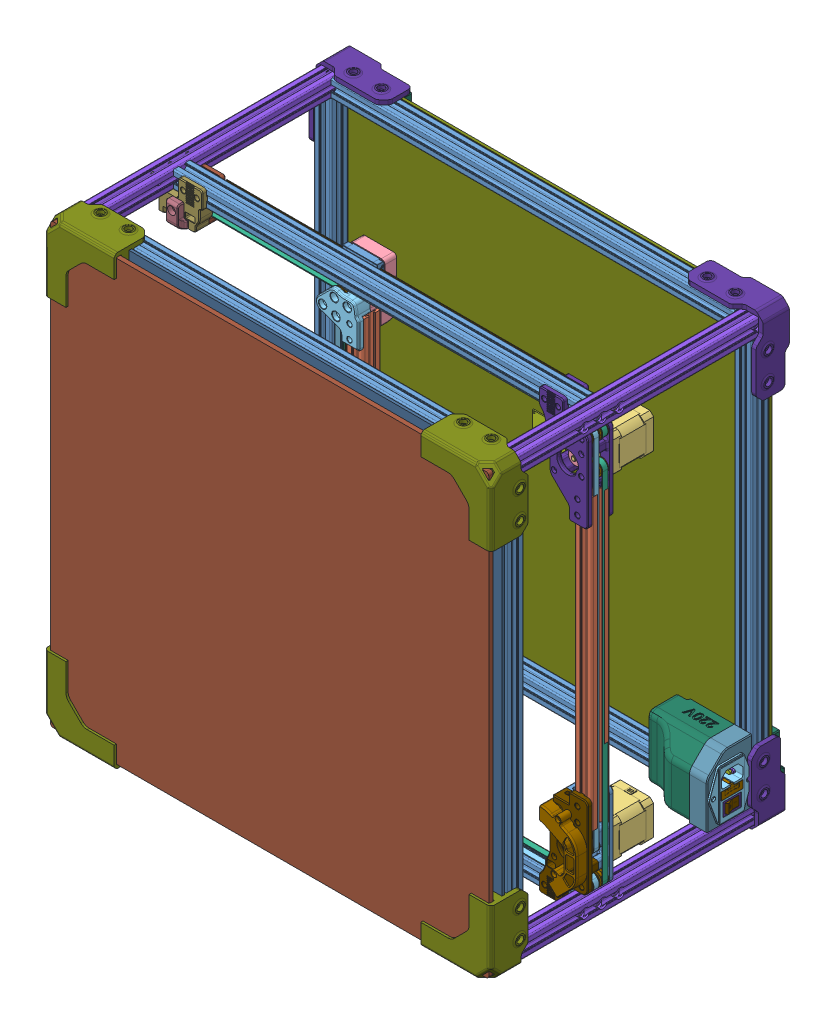
SolidWorks assembly Assem, configuration Default. Lengths in mm.
Overall size (512.11 512 340.5).
160 component instances, 72 part files, 301 mates.
Components (placement in the parent):
- ALP2020_460-1: ALP2020_460 [Default<As Machined>] at (0 240 0) size (460 20 20)
- ALP2020_460-2: ALP2020_460 [Default<As Machined>] at (0 -240 0) size (460 20 20)
- ALP2020_420-1: ALP2020_420 [Default<As Machined>] at (-23.2904 0 -0.3) x (0 1 0) z (0 0 1) size (420 20 20)
- XY Cable Chain Bridge - IGUS-58^XY Cable Chain Bridge - IGUS_XY Joint - Right_X Axis_Gantry_VORON2 v2.4 Assembly - Final(2)_VORON2 v2.4 Assembly - Final-1: XY Cable Chain Bridge - IGUS-58^XY Cable Chain Bridge - IGUS_XY Joint - Right_X Axis_Gantry_VORON2 v2.4 Assembly - Final(2)_VORON2 v2.4 Assembly - Final [Default] at (141.239 -208.6226 -52.6551) x (-1 0 0) z (0 0 1) size (21.02 66.15 41.04)
- XY Joint - Left-56^XY Joint - Left_X Axis_Gantry_VORON2 v2.4 Assembly - Final(2)_VORON2 v2.4 Assembly - Final-1: XY Joint - Left-56^XY Joint - Left_X Axis_Gantry_VORON2 v2.4 Assembly - Final(2)_VORON2 v2.4 Assembly - Final [Default] at (-39.2404 55.1999 -12.3) x (-1 0 0) z (0 0 1) size (49.35 57.43 34)
- XY Joint - Left-57^XY Joint - Left_X Axis_Gantry_VORON2 v2.4 Assembly - Final(2)_VORON2 v2.4 Assembly - Final-1: XY Joint - Left-57^XY Joint - Left_X Axis_Gantry_VORON2 v2.4 Assembly - Final(2)_VORON2 v2.4 Assembly - Final [Default] at (-39.2404 55.1999 -12.3) x (-1 0 0) z (0 0 1) size (49.07 51.45 16)
- XY Joint - Right-62^XY Joint - Right_X Axis_Gantry_VORON2 v2.4 Assembly - Final(2)_VORON2 v2.4 Assembly - Final-1: XY Joint - Right-62^XY Joint - Right_X Axis_Gantry_VORON2 v2.4 Assembly - Final(2)_VORON2 v2.4 Assembly - Final [Default] at (-39.2404 -250 -12.3) x (-1 0 0) z (0 0 1) size (49.07 51.45 16.71)
- XY Joint - Right-63^XY Joint - Right_X Axis_Gantry_VORON2 v2.4 Assembly - Final(2)_VORON2 v2.4 Assembly - Final-1: XY Joint - Right-63^XY Joint - Right_X Axis_Gantry_VORON2 v2.4 Assembly - Final(2)_VORON2 v2.4 Assembly - Final [Default] at (-39.2404 -250 -12.3) x (-1 0 0) z (0 0 1) size (49.23 57.43 34.01)
- GT2 20T Idler Gates v2^XY Joint - Right_X Axis_Gantry_VORON2 v2.4 Assembly - Final(2)_VORON2 v2.4 Assembly - Final-1: GT2 20T Idler Gates v2^XY Joint - Right_X Axis_Gantry_VORON2 v2.4 Assembly - Final(2)_VORON2 v2.4 Assembly - Final [Default] at (-53.9146 -207.89 -7) x (0 0 1) z (-0.999748 -0.022429 0) size (10 15 15)
- GT2 20T Idler Gates v2^XY Joint - Right_X Axis_Gantry_VORON2 v2.4 Assembly - Final(2)_VORON2 v2.4 Assembly - Final-2: GT2 20T Idler Gates v2^XY Joint - Right_X Axis_Gantry_VORON2 v2.4 Assembly - Final(2)_VORON2 v2.4 Assembly - Final [Default] at (-53.9146 207.89 -17) x (0 0 1) z (-0.999864 -0.01648 0) size (10 15 15)
- F695 ZZ (1)^Idler Assembly (1)_1_XY Joint - Right_X Axis_Gantry_VORON2 v2.4 Assembly - Final(2)_VORON2 v2.4 Assembly - Final-1: F695 ZZ (1)^Idler Assembly (1)_1_XY Joint - Right_X Axis_Gantry_VORON2 v2.4 Assembly - Final(2)_VORON2 v2.4 Assembly - Final [Default] at (-40.7546 -221.05 -9.3) x (1 0 0) z (0 -1 0) size (15 4 15)
- F695 ZZ (1)^Idler Assembly (1)_1_XY Joint - Right_X Axis_Gantry_VORON2 v2.4 Assembly - Final(2)_VORON2 v2.4 Assembly - Final-2: F695 ZZ (1)^Idler Assembly (1)_1_XY Joint - Right_X Axis_Gantry_VORON2 v2.4 Assembly - Final(2)_VORON2 v2.4 Assembly - Final [Default] at (-40.7546 -221.05 -1.3) x (-0.828596 0.559847 0) z (-0.559847 -0.828596 0) size (15 4 15)
- M5 1mm Spacer (1)^Idler Assembly (1)_1_XY Joint - Right_X Axis_Gantry_VORON2 v2.4 Assembly - Final(2)_VORON2 v2.4 Assembly - Final-1: M5 1mm Spacer (1)^Idler Assembly (1)_1_XY Joint - Right_X Axis_Gantry_VORON2 v2.4 Assembly - Final(2)_VORON2 v2.4 Assembly - Final [Default] at (-40.7546 -221.05 -10.4) size (10 10 1)
- M5 1mm Spacer (1)^Idler Assembly (1)_1_XY Joint - Right_X Axis_Gantry_VORON2 v2.4 Assembly - Final(2)_VORON2 v2.4 Assembly - Final-2: M5 1mm Spacer (1)^Idler Assembly (1)_1_XY Joint - Right_X Axis_Gantry_VORON2 v2.4 Assembly - Final(2)_VORON2 v2.4 Assembly - Final [Default] at (-40.7546 -221.05 -1.4) size (10 10 1)
- M5 1mm Spacer (1)^Idler Assembly (1)_1_XY Joint - Right_X Axis_Gantry_VORON2 v2.4 Assembly - Final(2)_VORON2 v2.4 Assembly - Final-3: M5 1mm Spacer (1)^Idler Assembly (1)_1_XY Joint - Right_X Axis_Gantry_VORON2 v2.4 Assembly - Final(2)_VORON2 v2.4 Assembly - Final [Default] at (-40.7546 221.05 8.6) size (10 10 1)
- M5 1mm Spacer (1)^Idler Assembly (1)_1_XY Joint - Right_X Axis_Gantry_VORON2 v2.4 Assembly - Final(2)_VORON2 v2.4 Assembly - Final-4: M5 1mm Spacer (1)^Idler Assembly (1)_1_XY Joint - Right_X Axis_Gantry_VORON2 v2.4 Assembly - Final(2)_VORON2 v2.4 Assembly - Final [Default] at (-40.7546 221.05 -0.4) size (10 10 1)
- F695 ZZ (1)^Idler Assembly (1)_1_XY Joint - Right_X Axis_Gantry_VORON2 v2.4 Assembly - Final(2)_VORON2 v2.4 Assembly - Final-3: F695 ZZ (1)^Idler Assembly (1)_1_XY Joint - Right_X Axis_Gantry_VORON2 v2.4 Assembly - Final(2)_VORON2 v2.4 Assembly - Final [Default] at (-40.7546 221.05 8.7) x (-0.825451 0.564473 0) z (-0.564473 -0.825451 0) size (15 4 15)
- F695 ZZ (1)^Idler Assembly (1)_1_XY Joint - Right_X Axis_Gantry_VORON2 v2.4 Assembly - Final(2)_VORON2 v2.4 Assembly - Final-4: F695 ZZ (1)^Idler Assembly (1)_1_XY Joint - Right_X Axis_Gantry_VORON2 v2.4 Assembly - Final(2)_VORON2 v2.4 Assembly - Final [Default] at (-40.7546 221.05 0.7) x (1 0 0) z (0 -1 0) size (15 4 15)
- Front Idler B Bottom^Front Idler B_Gantry_VORON2 v2.4 Assembly - Final(2)_VORON2 v2.4 Assembly - Final-1: Front Idler B Bottom^Front Idler B_Gantry_VORON2 v2.4 Assembly - Final(2)_VORON2 v2.4 Assembly - Final [Default] at (137.5068 690.5733 49.206) x (-1 0 0) z (0 0 -1) size (50.59 46.02 19.26)
- Front Idler B Top^Front Idler B_Gantry_VORON2 v2.4 Assembly - Final(2)_VORON2 v2.4 Assembly - Final-1: Front Idler B Top^Front Idler B_Gantry_VORON2 v2.4 Assembly - Final(2)_VORON2 v2.4 Assembly - Final [Default] at (137.5068 -292.5733 -49.0508) x (-1 0 0) z (0 0 1) size (52.55 46.03 19.69)
- Tensioner B-26^Tensioner B_Front Idler B_Gantry_VORON2 v2.4 Assembly - Final(2)_VORON2 v2.4 Assembly - Final-1: Tensioner B-26^Tensioner B_Front Idler B_Gantry_VORON2 v2.4 Assembly - Final(2)_VORON2 v2.4 Assembly - Final [Default] at (137.5068 500.5733 49.406) x (-1 0 0) z (0 0 -1) size (18 25.05 45.03)
- M5 1mm Spacer (1)^Idler Assembly (1)_1_XY Joint - Right_X Axis_Gantry_VORON2 v2.4 Assembly - Final(2)_VORON2 v2.4 Assembly - Final-5: M5 1mm Spacer (1)^Idler Assembly (1)_1_XY Joint - Right_X Axis_Gantry_VORON2 v2.4 Assembly - Final(2)_VORON2 v2.4 Assembly - Final [Default] at (-219.5002 221.0003 -8.9) x (0.890393 0.455193 0) z (0 0 -1) size (10 10 1)
- F695 ZZ (1)^Idler Assembly (1)_1_XY Joint - Right_X Axis_Gantry_VORON2 v2.4 Assembly - Final(2)_VORON2 v2.4 Assembly - Final-5: F695 ZZ (1)^Idler Assembly (1)_1_XY Joint - Right_X Axis_Gantry_VORON2 v2.4 Assembly - Final(2)_VORON2 v2.4 Assembly - Final [Default] at (-219.5002 221.0003 -1) x (0.923728 0.383049 0) z (-0.383049 0.923728 0) size (15 4 15)
- F695 ZZ (1)^Idler Assembly (1)_1_XY Joint - Right_X Axis_Gantry_VORON2 v2.4 Assembly - Final(2)_VORON2 v2.4 Assembly - Final-6: F695 ZZ (1)^Idler Assembly (1)_1_XY Joint - Right_X Axis_Gantry_VORON2 v2.4 Assembly - Final(2)_VORON2 v2.4 Assembly - Final [Default] at (-219.5002 221.0003 -9) x (-0.593635 -0.804734 0) z (-0.804734 0.593635 0) size (15 4 15)
- M5 1mm Spacer (1)^Idler Assembly (1)_1_XY Joint - Right_X Axis_Gantry_VORON2 v2.4 Assembly - Final(2)_VORON2 v2.4 Assembly - Final-6: M5 1mm Spacer (1)^Idler Assembly (1)_1_XY Joint - Right_X Axis_Gantry_VORON2 v2.4 Assembly - Final(2)_VORON2 v2.4 Assembly - Final [Default] at (-219.5002 221.0003 0.1) x (0.923728 0.383049 0) z (0 0 -1) size (10 10 1)
- Front Idler A Bottom (1)^Front Idler A_Gantry_VORON2 v2.4 Assembly - Final(2)_VORON2 v2.4 Assembly - Final-1: Front Idler A Bottom (1)^Front Idler A_Gantry_VORON2 v2.4 Assembly - Final(2)_VORON2 v2.4 Assembly - Final [Default] at (137.5068 -500.5733 -20.406) x (-1 0 0) z (0 0 1) size (50.59 46.03 18.86)
- Front Idler A Top^Front Idler A_Gantry_VORON2 v2.4 Assembly - Final(2)_VORON2 v2.4 Assembly - Final-1: Front Idler A Top^Front Idler A_Gantry_VORON2 v2.4 Assembly - Final(2)_VORON2 v2.4 Assembly - Final [Default] at (137.5068 96.5732 20.406) x (-1 0 0) z (0 0 -1) size (52.55 46.02 19.26)
- Tensioner A-25^Tensioner A_Front Idler A_Gantry_VORON2 v2.4 Assembly - Final(2)_VORON2 v2.4 Assembly - Final-1: Tensioner A-25^Tensioner A_Front Idler A_Gantry_VORON2 v2.4 Assembly - Final(2)_VORON2 v2.4 Assembly - Final [Default] at (-219.5002 -221.0003 1) x (-1 0 0) z (0 1 0) size (18 45.03 25.05)
- M5 1mm Spacer (1)^Idler Assembly (1)_1_XY Joint - Right_X Axis_Gantry_VORON2 v2.4 Assembly - Final(2)_VORON2 v2.4 Assembly - Final-7: M5 1mm Spacer (1)^Idler Assembly (1)_1_XY Joint - Right_X Axis_Gantry_VORON2 v2.4 Assembly - Final(2)_VORON2 v2.4 Assembly - Final [Default] at (-219.5002 -221.0003 10.1) x (0.923728 0.383049 0) z (0 0 -1) size (10 10 1)
- F695 ZZ (1)^Idler Assembly (1)_1_XY Joint - Right_X Axis_Gantry_VORON2 v2.4 Assembly - Final(2)_VORON2 v2.4 Assembly - Final-7: F695 ZZ (1)^Idler Assembly (1)_1_XY Joint - Right_X Axis_Gantry_VORON2 v2.4 Assembly - Final(2)_VORON2 v2.4 Assembly - Final [Default] at (-219.5002 -221.0003 1) x (-0.56381 -0.825904 0) z (-0.825904 0.56381 0) size (15 4 15)
- F695 ZZ (1)^Idler Assembly (1)_1_XY Joint - Right_X Axis_Gantry_VORON2 v2.4 Assembly - Final(2)_VORON2 v2.4 Assembly - Final-8: F695 ZZ (1)^Idler Assembly (1)_1_XY Joint - Right_X Axis_Gantry_VORON2 v2.4 Assembly - Final(2)_VORON2 v2.4 Assembly - Final [Default] at (-219.5002 -221.0003 9) x (0.923728 0.383049 0) z (-0.383049 0.923728 0) size (15 4 15)
- M5 1mm Spacer (1)^Idler Assembly (1)_1_XY Joint - Right_X Axis_Gantry_VORON2 v2.4 Assembly - Final(2)_VORON2 v2.4 Assembly - Final-8: M5 1mm Spacer (1)^Idler Assembly (1)_1_XY Joint - Right_X Axis_Gantry_VORON2 v2.4 Assembly - Final(2)_VORON2 v2.4 Assembly - Final [Default] at (-219.5002 -221.0003 1.1) x (0.923728 0.383049 0) z (0 0 -1) size (10 10 1)
- B Drive Frame (1)^B Drive_Gantry_VORON2 v2.4 Assembly - Final(2)_VORON2 v2.4 Assembly - Final-1: B Drive Frame (1)^B Drive_Gantry_VORON2 v2.4 Assembly - Final(2)_VORON2 v2.4 Assembly - Final [Default] at (227.5294 207.0226 -33.306) x (-1 0 0) z (0 0 -1) size (56.03 116 32.01)
- A Drive Frame-23^A Drive Frame_A Drive_Gantry_VORON2 v2.4 Assembly - Final(2)_VORON2 v2.4 Assembly - Final-1: A Drive Frame-23^A Drive Frame_A Drive_Gantry_VORON2 v2.4 Assembly - Final(2)_VORON2 v2.4 Assembly - Final [Default] at (227.5294 -207.0226 -33.306) x (-1 0 0) z (0 0 1) size (56.03 116 16.01)
- A Drive Frame-24^A Drive Frame_A Drive_Gantry_VORON2 v2.4 Assembly - Final(2)_VORON2 v2.4 Assembly - Final-1: A Drive Frame-24^A Drive Frame_A Drive_Gantry_VORON2 v2.4 Assembly - Final(2)_VORON2 v2.4 Assembly - Final [Default] at (227.5294 -207.0226 -33.306) x (-1 0 0) z (0 0 1) size (53.03 116 18.01)
- ALP2020_330-1: ALP2020_330 [Default<As Machined>] at (238.0294 -0.0226 0) x (0 1 0) z (0 0 1) size (330 20 20)
- M5 1mm Spacer (1)^Idler Assembly (1)_1_XY Joint - Right_X Axis_Gantry_VORON2 v2.4 Assembly - Final(2)_VORON2 v2.4 Assembly - Final-9: M5 1mm Spacer (1)^Idler Assembly (1)_1_XY Joint - Right_X Axis_Gantry_VORON2 v2.4 Assembly - Final(2)_VORON2 v2.4 Assembly - Final [Default] at (240.5294 -221.1733 1.1) x (0.923728 0.383049 0) z (0 0 -1) size (10 10 1)
- F695 ZZ (1)^Idler Assembly (1)_1_XY Joint - Right_X Axis_Gantry_VORON2 v2.4 Assembly - Final(2)_VORON2 v2.4 Assembly - Final-9: F695 ZZ (1)^Idler Assembly (1)_1_XY Joint - Right_X Axis_Gantry_VORON2 v2.4 Assembly - Final(2)_VORON2 v2.4 Assembly - Final [Default] at (240.5294 -221.1733 9) x (0.923728 0.383049 0) z (-0.383049 0.923728 0) size (15 4 15)
- F695 ZZ (1)^Idler Assembly (1)_1_XY Joint - Right_X Axis_Gantry_VORON2 v2.4 Assembly - Final(2)_VORON2 v2.4 Assembly - Final-10: F695 ZZ (1)^Idler Assembly (1)_1_XY Joint - Right_X Axis_Gantry_VORON2 v2.4 Assembly - Final(2)_VORON2 v2.4 Assembly - Final [Default] at (240.5294 -221.1733 1) x (-0.56381 -0.825904 0) z (-0.825904 0.56381 0) size (15 4 15)
- M5 1mm Spacer (1)^Idler Assembly (1)_1_XY Joint - Right_X Axis_Gantry_VORON2 v2.4 Assembly - Final(2)_VORON2 v2.4 Assembly - Final-10: M5 1mm Spacer (1)^Idler Assembly (1)_1_XY Joint - Right_X Axis_Gantry_VORON2 v2.4 Assembly - Final(2)_VORON2 v2.4 Assembly - Final [Default] at (240.5294 -221.1733 10.1) x (0.923728 0.383049 0) z (0 0 -1) size (10 10 1)
- M5 1mm Spacer (1)^Idler Assembly (1)_1_XY Joint - Right_X Axis_Gantry_VORON2 v2.4 Assembly - Final(2)_VORON2 v2.4 Assembly - Final-11: M5 1mm Spacer (1)^Idler Assembly (1)_1_XY Joint - Right_X Axis_Gantry_VORON2 v2.4 Assembly - Final(2)_VORON2 v2.4 Assembly - Final [Default] at (240.5294 -221.1733 0.1) x (0.923728 0.383049 0) z (0 0 -1) size (10 10 1)
- F695 ZZ (1)^Idler Assembly (1)_1_XY Joint - Right_X Axis_Gantry_VORON2 v2.4 Assembly - Final(2)_VORON2 v2.4 Assembly - Final-11: F695 ZZ (1)^Idler Assembly (1)_1_XY Joint - Right_X Axis_Gantry_VORON2 v2.4 Assembly - Final(2)_VORON2 v2.4 Assembly - Final [Default] at (240.5294 -221.1733 -9) x (-0.56381 -0.825904 0) z (-0.825904 0.56381 0) size (15 4 15)
- F695 ZZ (1)^Idler Assembly (1)_1_XY Joint - Right_X Axis_Gantry_VORON2 v2.4 Assembly - Final(2)_VORON2 v2.4 Assembly - Final-12: F695 ZZ (1)^Idler Assembly (1)_1_XY Joint - Right_X Axis_Gantry_VORON2 v2.4 Assembly - Final(2)_VORON2 v2.4 Assembly - Final [Default] at (240.5294 -221.1733 -1) x (0.929551 0.368694 0) z (-0.368694 0.929551 0) size (15 4 15)
- M5 1mm Spacer (1)^Idler Assembly (1)_1_XY Joint - Right_X Axis_Gantry_VORON2 v2.4 Assembly - Final(2)_VORON2 v2.4 Assembly - Final-12: M5 1mm Spacer (1)^Idler Assembly (1)_1_XY Joint - Right_X Axis_Gantry_VORON2 v2.4 Assembly - Final(2)_VORON2 v2.4 Assembly - Final [Default] at (240.5294 -221.1733 -8.9) x (0.923728 0.383049 0) z (0 0 -1) size (10 10 1)
- M5 1mm Spacer (1)^Idler Assembly (1)_1_XY Joint - Right_X Axis_Gantry_VORON2 v2.4 Assembly - Final(2)_VORON2 v2.4 Assembly - Final-13: M5 1mm Spacer (1)^Idler Assembly (1)_1_XY Joint - Right_X Axis_Gantry_VORON2 v2.4 Assembly - Final(2)_VORON2 v2.4 Assembly - Final [Default] at (240.5294 221.1733 -8.9) x (0.923728 0.383049 0) z (0 0 -1) size (10 10 1)
- F695 ZZ (1)^Idler Assembly (1)_1_XY Joint - Right_X Axis_Gantry_VORON2 v2.4 Assembly - Final(2)_VORON2 v2.4 Assembly - Final-13: F695 ZZ (1)^Idler Assembly (1)_1_XY Joint - Right_X Axis_Gantry_VORON2 v2.4 Assembly - Final(2)_VORON2 v2.4 Assembly - Final [Default] at (240.5294 221.1733 -1) x (0.937118 0.349013 0) z (-0.349013 0.937118 0) size (15 4 15)
- F695 ZZ (1)^Idler Assembly (1)_1_XY Joint - Right_X Axis_Gantry_VORON2 v2.4 Assembly - Final(2)_VORON2 v2.4 Assembly - Final-14: F695 ZZ (1)^Idler Assembly (1)_1_XY Joint - Right_X Axis_Gantry_VORON2 v2.4 Assembly - Final(2)_VORON2 v2.4 Assembly - Final [Default] at (240.5294 221.1733 -9) x (-0.56381 -0.825904 0) z (-0.825904 0.56381 0) size (15 4 15)
- M5 1mm Spacer (1)^Idler Assembly (1)_1_XY Joint - Right_X Axis_Gantry_VORON2 v2.4 Assembly - Final(2)_VORON2 v2.4 Assembly - Final-14: M5 1mm Spacer (1)^Idler Assembly (1)_1_XY Joint - Right_X Axis_Gantry_VORON2 v2.4 Assembly - Final(2)_VORON2 v2.4 Assembly - Final [Default] at (240.5294 221.1733 0.1) x (0.923728 0.383049 0) z (0 0 -1) size (10 10 1)
- M5 1mm Spacer (1)^Idler Assembly (1)_1_XY Joint - Right_X Axis_Gantry_VORON2 v2.4 Assembly - Final(2)_VORON2 v2.4 Assembly - Final-15: M5 1mm Spacer (1)^Idler Assembly (1)_1_XY Joint - Right_X Axis_Gantry_VORON2 v2.4 Assembly - Final(2)_VORON2 v2.4 Assembly - Final [Default] at (240.5294 221.1733 10.1) x (0.923728 0.383049 0) z (0 0 -1) size (10 10 1)
- F695 ZZ (1)^Idler Assembly (1)_1_XY Joint - Right_X Axis_Gantry_VORON2 v2.4 Assembly - Final(2)_VORON2 v2.4 Assembly - Final-15: F695 ZZ (1)^Idler Assembly (1)_1_XY Joint - Right_X Axis_Gantry_VORON2 v2.4 Assembly - Final(2)_VORON2 v2.4 Assembly - Final [Default] at (240.5294 221.1733 1) x (-0.777057 -0.62943 0) z (-0.62943 0.777057 0) size (15 4 15)
- F695 ZZ (1)^Idler Assembly (1)_1_XY Joint - Right_X Axis_Gantry_VORON2 v2.4 Assembly - Final(2)_VORON2 v2.4 Assembly - Final-16: F695 ZZ (1)^Idler Assembly (1)_1_XY Joint - Right_X Axis_Gantry_VORON2 v2.4 Assembly - Final(2)_VORON2 v2.4 Assembly - Final [Default] at (240.5294 221.1733 9) x (0.923728 0.383049 0) z (-0.383049 0.923728 0) size (15 4 15)
- M5 1mm Spacer (1)^Idler Assembly (1)_1_XY Joint - Right_X Axis_Gantry_VORON2 v2.4 Assembly - Final(2)_VORON2 v2.4 Assembly - Final-16: M5 1mm Spacer (1)^Idler Assembly (1)_1_XY Joint - Right_X Axis_Gantry_VORON2 v2.4 Assembly - Final(2)_VORON2 v2.4 Assembly - Final [Default] at (240.5294 221.1733 1.1) x (0.923728 0.383049 0) z (0 0 -1) size (10 10 1)
- M5 1mm Spacer (1)^Idler Assembly (1)_1_XY Joint - Right_X Axis_Gantry_VORON2 v2.4 Assembly - Final(2)_VORON2 v2.4 Assembly - Final-17: M5 1mm Spacer (1)^Idler Assembly (1)_1_XY Joint - Right_X Axis_Gantry_VORON2 v2.4 Assembly - Final(2)_VORON2 v2.4 Assembly - Final [Default] at (240.5064 184.1733 -8.9) x (0.923728 0.383049 0) z (0 0 -1) size (10 10 1)
- F695 ZZ (1)^Idler Assembly (1)_1_XY Joint - Right_X Axis_Gantry_VORON2 v2.4 Assembly - Final(2)_VORON2 v2.4 Assembly - Final-17: F695 ZZ (1)^Idler Assembly (1)_1_XY Joint - Right_X Axis_Gantry_VORON2 v2.4 Assembly - Final(2)_VORON2 v2.4 Assembly - Final [Default] at (240.5064 184.1733 -1) x (0.923728 0.383049 0) z (-0.383049 0.923728 0) size (15 4 15)
- F695 ZZ (1)^Idler Assembly (1)_1_XY Joint - Right_X Axis_Gantry_VORON2 v2.4 Assembly - Final(2)_VORON2 v2.4 Assembly - Final-18: F695 ZZ (1)^Idler Assembly (1)_1_XY Joint - Right_X Axis_Gantry_VORON2 v2.4 Assembly - Final(2)_VORON2 v2.4 Assembly - Final [Default] at (240.5064 184.1733 -9) x (-0.576536 -0.817071 0) z (-0.817071 0.576536 0) size (15 4 15)
- M5 1mm Spacer (1)^Idler Assembly (1)_1_XY Joint - Right_X Axis_Gantry_VORON2 v2.4 Assembly - Final(2)_VORON2 v2.4 Assembly - Final-18: M5 1mm Spacer (1)^Idler Assembly (1)_1_XY Joint - Right_X Axis_Gantry_VORON2 v2.4 Assembly - Final(2)_VORON2 v2.4 Assembly - Final [Default] at (240.5064 184.1733 0.1) x (0.923728 0.383049 0) z (0 0 -1) size (10 10 1)
- M5 1mm Spacer (1)^Idler Assembly (1)_1_XY Joint - Right_X Axis_Gantry_VORON2 v2.4 Assembly - Final(2)_VORON2 v2.4 Assembly - Final-19: M5 1mm Spacer (1)^Idler Assembly (1)_1_XY Joint - Right_X Axis_Gantry_VORON2 v2.4 Assembly - Final(2)_VORON2 v2.4 Assembly - Final [Default] at (240.5064 -184.1733 10.1) x (0.923728 0.383049 0) z (0 0 -1) size (10 10 1)
- F695 ZZ (1)^Idler Assembly (1)_1_XY Joint - Right_X Axis_Gantry_VORON2 v2.4 Assembly - Final(2)_VORON2 v2.4 Assembly - Final-19: F695 ZZ (1)^Idler Assembly (1)_1_XY Joint - Right_X Axis_Gantry_VORON2 v2.4 Assembly - Final(2)_VORON2 v2.4 Assembly - Final [Default] at (240.5064 -184.1733 1) x (-0.581098 -0.813834 0) z (-0.813834 0.581098 0) size (15 4 15)
- F695 ZZ (1)^Idler Assembly (1)_1_XY Joint - Right_X Axis_Gantry_VORON2 v2.4 Assembly - Final(2)_VORON2 v2.4 Assembly - Final-20: F695 ZZ (1)^Idler Assembly (1)_1_XY Joint - Right_X Axis_Gantry_VORON2 v2.4 Assembly - Final(2)_VORON2 v2.4 Assembly - Final [Default] at (240.5064 -184.1733 9) x (0.923728 0.383049 0) z (-0.383049 0.923728 0) size (15 4 15)
- M5 1mm Spacer (1)^Idler Assembly (1)_1_XY Joint - Right_X Axis_Gantry_VORON2 v2.4 Assembly - Final(2)_VORON2 v2.4 Assembly - Final-20: M5 1mm Spacer (1)^Idler Assembly (1)_1_XY Joint - Right_X Axis_Gantry_VORON2 v2.4 Assembly - Final(2)_VORON2 v2.4 Assembly - Final [Default] at (240.5064 -184.1733 1.1) x (0.923728 0.383049 0) z (0 0 -1) size (10 10 1)
- NEMA17 Black^B Drive_Gantry_VORON2 v2.4 Assembly - Final(2)_VORON2 v2.4 Assembly - Final-1: NEMA17 Black^B Drive_Gantry_VORON2 v2.4 Assembly - Final(2)_VORON2 v2.4 Assembly - Final [Default] at (225.0294 190.9774 -33.56) size (42.2 42.61 70.85)
- NEMA17 Black^B Drive_Gantry_VORON2 v2.4 Assembly - Final(2)_VORON2 v2.4 Assembly - Final-2: NEMA17 Black^B Drive_Gantry_VORON2 v2.4 Assembly - Final(2)_VORON2 v2.4 Assembly - Final [Default] at (225.0294 -190.9774 -33.56) x (-1 0 0) z (0 0 1) size (42.2 42.61 70.85)
- GT2 20T 6mm^B Drive_Gantry_VORON2 v2.4 Assembly - Final(2)_VORON2 v2.4 Assembly - Final-1: GT2 20T 6mm^B Drive_Gantry_VORON2 v2.4 Assembly - Final(2)_VORON2 v2.4 Assembly - Final [Default] at (225.0294 -190.9774 -6.35) x (0 0 1) z (-0.999748 -0.022429 0) size (16 16 16)
- GT2 20T 6mm^B Drive_Gantry_VORON2 v2.4 Assembly - Final(2)_VORON2 v2.4 Assembly - Final-2: GT2 20T 6mm^B Drive_Gantry_VORON2 v2.4 Assembly - Final(2)_VORON2 v2.4 Assembly - Final [Default] at (225.0294 190.9774 6.35) x (0 0 -1) z (0.91729 0.39822 0) size (16 16 16)
- Belt2-4-1: Belt2-4 [Default] at (220.0294 -190.9774 5) x (-1 0 0) z (0 0 -1) size (474.81 457.12 6.02)
- Belt1-5-1: Belt1-5 [Default] at (220.0294 190.9774 -5) size (475.05 457.36 6)
- ALP2020_460-3: ALP2020_460 [Default<As Machined>] at (0 240 100) size (460 20 20)
- ALP2020_460-4: ALP2020_460 [Default<As Machined>] at (-240 0 100) x (0 -1 0) z (0 0 1) size (460 20 20)
- ALP2020_460-5: ALP2020_460 [Default<As Machined>] at (240 0 100) x (0 -1 0) z (0 0 1) size (460 20 20)
- ALP2020_460-6: ALP2020_460 [Default<As Machined>] at (0 -240 100) size (460 20 20)
- ALP2020_460-7: ALP2020_460 [Default<As Machined>] at (-240 0 -180) x (0 -1 0) z (0 0 1) size (460 20 20)
- ALP2020_460-8: ALP2020_460 [Default<As Machined>] at (0 -240 -180) size (460 20 20)
- ALP2020_460-9: ALP2020_460 [Default<As Machined>] at (240 0 -180) x (0 -1 0) z (0 0 1) size (460 20 20)
- ALP2020_460-10: ALP2020_460 [Default<As Machined>] at (0 240 -180) size (460 20 20)
- camera-1: camera [默认] at (-5.0058 -4.6135 -190) x (0 1 0) z (1 0 0) size (38 18.6 38)
- ALP2020_300-1: ALP2020_300 [Default<As Machined>] at (-240 -240 -40) size (20 20 300)
- ALP2020_300-2: ALP2020_300 [Default<As Machined>] at (-240 240 -40) size (20 20 300)
- ALP2020_300-4: ALP2020_300 [Default<As Machined>] at (240 -240 -40) x (-1 0 0) z (0 0 1) size (20 20 300)
- ALP2020_300-5: ALP2020_300 [Default<As Machined>] at (240 240 -40) x (-1 0 0) z (0 0 1) size (20 20 300)
- cable cover^A Drive_Gantry_VORON2 v2.4 Assembly - Final(2)_VORON2 v2.4 Assembly - Final-1: cable cover^A Drive_Gantry_VORON2 v2.4 Assembly - Final(2)_VORON2 v2.4 Assembly - Final [Default] at (-122.0004 82 -44) x (0 -1 0) z (0 0 1) size (82.16 43 35.3)
- GlassSheet3mm-1: GlassSheet3mm [Default] at (0 0 115) x (1 0 0) z (0 1 0) size (500 3 500)
- GlassSheet5mm-1: GlassSheet5mm [Default] at (0 0 130) x (1 0 0) z (0 1 0) size (500 5 500)
- X Carriage Frame-36^X Carriage Frame_X Carriage_X Axis_Gantry_VORON2 v2.4 Assembly - Final(2)_VORON2 v2.4 Assembly - Final-1: X Carriage Frame-36^X Carriage Frame_X Carriage_X Axis_Gantry_VORON2 v2.4 Assembly - Final(2)_VORON2 v2.4 Assembly - Final [Default] at (-106.1195 89.2516 -13.1137) x (-1 0 0) z (0 0 1) size (26.65 20 66.75)
- X Carriage Frame-35^X Carriage Frame_X Carriage_X Axis_Gantry_VORON2 v2.4 Assembly - Final(2)_VORON2 v2.4 Assembly - Final-1: X Carriage Frame-35^X Carriage Frame_X Carriage_X Axis_Gantry_VORON2 v2.4 Assembly - Final(2)_VORON2 v2.4 Assembly - Final [Default] at (-106.1195 89.2516 -13.1137) x (-1 0 0) z (0 0 1) size (26.6 22 66.75)
- Belt Clamp_1-34^Belt Clamp_1_X Carriage Frame_X Carriage_X Axis_Gantry_VORON2 v2.4 Assembly - Final(2)_VORON2 v2.4 Assembly - Final-1: Belt Clamp_1-34^Belt Clamp_1_X Carriage Frame_X Carriage_X Axis_Gantry_VORON2 v2.4 Assembly - Final(2)_VORON2 v2.4 Assembly - Final [Default] at (170.339 -77.2136 -115.3) x (-1 0 0) z (0 0 1) size (8.63 6.1 15.9)
- FootCorner-1: FootCorner [Default] at (-230 230 -193) x (0 1 0) z (-1 0 0) size (80 15 80)
- FootCorner-2: FootCorner [Default] at (230 230 -193) x (1 0 0) z (0 1 0) size (80 15 80)
- FootCorner-3: FootCorner [Default] at (-230 -230 -193) x (-1 0 0) z (0 -1 0) size (80 15 80)
- FootCorner-4: FootCorner [Default] at (230 -230 -193) x (0 -1 0) z (1 0 0) size (80 15 80)
- BottomAcrylicPanel-1: BottomAcrylicPanel [Default] at (0 240 -190) x (-1 0 0) z (0 0 -1) size (500 500 3)
- IEC320-C14-1: IEC320-C14 [Default] at (288.0045 -231.951 -173.0106) x (0 0 1) z (-1 0 0) size (49.49 57.9 32.67)
  - IEC320-C14.STEP-1: IEC320-C14.STEP [Default] at origin size (49.49 57.9 32.67)
    - switch.STEP-1: switch.STEP [Default] at (42.0854 20.5719 65.6615) x (0 -1 0) z (0 0 -1) size (14.95 21.3 26.46)
      - switch_base.STEP-1: switch_base.STEP [Default] at (1.8459 13.5998 28.607) size (14.95 21.3 22.44)
      - rocker.STEP-1: rocker.STEP [Default] at (-3.4041 13.6325 27.5754) x (1 0 0) z (0 -0.190809 -0.981627) size (12.5 17 8.39)
      - sm_tab_type1a.STEP-1: sm_tab_type1a.STEP [Default] at (-2.0041 15.2392 15.457) x (0 1 0) z (-1 0 0) size (5.64 8.55 2.63)
      - sm_tab_type1b.STEP-1: sm_tab_type1b.STEP [Default] at (4.5038 6.6165 15.457) x (0 1 0) z (-1 0 0) size (5.64 8.55 2.63)
      - sm_tab_type2a.STEP-1: sm_tab_type2a.STEP [Default] at (5.6959 20.212 15.457) x (0 -1 0) z (1 0 0) size (4.75 8.55 2.63)
      - sm_tab_type2b.STEP-1: sm_tab_type2b.STEP [Default] at (-0.812 11.2545 15.457) x (0 -1 0) z (1 0 0) size (4.75 8.55 2.63)
    - ilpm_case.STEP-1: ilpm_case.STEP [Default] at (28.5106 33.401 38.0045) size (49.49 57.9 24.2)
    - fuse_clip_set.STEP-1: fuse_clip_set.STEP [Default] at (28.5106 32.951 54.6045) x (1 0 0) z (0 1 0) size (21.11 9.2 8)
    - blade_15.STEP-1: blade_15.STEP [Default] at (27.5106 49.451 52.4045) x (0 -1 0) z (1 0 0) size (5.25 21.2 2.8)
    - blade_12.STEP-1: blade_12.STEP [Default] at (34.5106 45.451 52.4045) x (0 -1 0) z (1 0 0) size (5.25 18.2 2.8)
    - blade_12.STEP-2: blade_12.STEP [Default] at (20.5106 45.451 52.4045) x (0 -1 0) z (1 0 0) size (5.25 18.2 2.8)
    - fuse-holder.STEP-1: fuse-holder.STEP [Default] at (40.8606 32.851 39.1545) x (0 1 0) z (-1 0 0) size (12.5 19.58 24.7)
    - fuse.STEP-1: fuse.STEP [Default] at (37.5106 32.8033 47.1545) x (0 0 1) z (-1 0 0) size (4.97 4.97 20)
    - spot.STEP-1: spot.STEP [Default] at (20.346 31.435 52.5045) x (1 0 0) z (0 1 0) size (2.8 2 2.8)
    - spot.STEP-2: spot.STEP [Default] at (37.2713 31.435 52.5045) x (1 0 0) z (0 1 0) size (2.8 2 2.8)
    - stamped_cond.STEP-1: stamped_cond.STEP [Default] at (32.3106 42.901 55.5045) size (6.4 19.8 0.5)
    - correct_big_tab.STEP-1: correct_big_tab.STEP [Default] at (18.3106 42.841 56.3545) x (1 0 0) z (0 -1 0) size (6.3 9 6)
    - correct_big_tab.STEP-2: correct_big_tab.STEP [Default] at (31.6106 51.861 56.3545) x (-1 0 0) z (0 1 0) size (6.3 9 6)
    - correct_big_tab.STEP-3: correct_big_tab.STEP [Default] at (17.0606 30.053 56.3545) x (1 0 0) z (0 -1 0) size (6.3 9 6)
- PowerSwitchMount-1: PowerSwitchMount [Default] at (250 -198.55 -144.5) x (0 0 1) z (-1 0 0) size (51 72 20)
- PowerCover-1: PowerCover [Default] at (230 -198.55 -144.5) x (0 0 1) z (-1 0 0) size (51 72 65.28)
- GlassSheetHolderCorner2-1: GlassSheetHolderCorner2 [Default] at (-230 -230 110) x (0 -1 0) z (-1 0 0) size (81 42.5 81)
- BottomCorner-1: BottomCorner [Default] at (-250 0 -180) x (0 1 0) z (-1 0 0) size (86 38 86)
- BottomCorner-2: BottomCorner [Default] at (0 -250 -175) x (-1 0 0) z (0 -1 0) size (86 38 86)
- GlassSheetHolderCorner2-2: GlassSheetHolderCorner2 [Default] at (230 -230 110) x (1 0 0) z (0 -1 0) size (81 42.5 81)
- GlassSheetHolderCorner2-3: GlassSheetHolderCorner2 [Default] at (-230 230 110) x (-1 0 0) z (0 1 0) size (81 42.5 81)
- GlassSheetHolderCorner2-4: GlassSheetHolderCorner2 [Default] at (230 230 110) x (0 1 0) z (1 0 0) size (81 42.5 81)
- BottomCorner-3: BottomCorner [Default] at (250 0 -180) x (0 -1 0) z (1 0 0) size (86 38 86)
- BottomCorner-4: BottomCorner [Default] at (0 250 -180) x (1 0 0) z (0 1 0) size (86 38 86)
- MGN9-390-1: MGN9-390 [По умолчанию] at (-195 240 -13.25) x (0 -1 0) z (1 0 0) size (20 10 390)
  - MGN9-1: MGN9 [По умолчанию] at origin size (9 6.5 390)
  - MGN9-H-1: MGN9-H [По умолчанию] at (0 2.75 155.8096) size (20 8 40.67)
- MGN9-390-2: MGN9-390 [По умолчанию] at (-195 -240 -13.25) x (0 -1 0) z (1 0 0) size (20 10 390)
  - MGN9-1: MGN9 [По умолчанию] at origin size (9 6.5 390)
  - MGN9-H-1: MGN9-H [По умолчанию] at (0 2.75 155.8096) size (20 8 40.67)
- MGN9-390-3: MGN9-390 [По умолчанию] at (-36.5404 -195.1 -0.3) x (0 0 -1) z (0 1 0) size (20 10 390)
  - MGN9-1: MGN9 [По умолчанию] at origin size (9 6.5 390)
  - MGN9-H-1: MGN9-H [По умолчанию] at (0 2.75 155.8096) size (20 8 40.67)
- Belt Clamp_1-34^Belt Clamp_1_X Carriage Frame_X Carriage_X Axis_Gantry_VORON2 v2.4 Assembly - Final(2)_VORON2 v2.4 Assembly - Final-2: Belt Clamp_1-34^Belt Clamp_1_X Carriage Frame_X Carriage_X Axis_Gantry_VORON2 v2.4 Assembly - Final(2)_VORON2 v2.4 Assembly - Final [Default] at (-280.9198 -1.3672 -115.3) size (8.63 6.1 15.9)
- CoilBase-1: CoilBase [Default] at (-41.9766 -3.9237 115) x (1 0 0) z (0 -1 0) size (60 8 60)
- T8LeadScrew-1: T8LeadScrew [Default] at (-57.6904 -39.2904 -23) x (1 0 0) z (0 -1 0) size (30.45 116.78 30.45) (flexible)
  - 8mm trapez mil-1: 8mm trapez mil [Varsayılan] at origin size (8.11 116.78 9.24)
  - T8 nut-1: T8 nut [Default] at (0 83.7422 0) x (-0.837169 0 -0.546944) z (0 1 0) size (22 22 15)
- D20L25 Jaw Coupler v5-1: D20L25 Jaw Coupler v5 [Default] at (-57.6904 -39.2904 -38.1704) x (-0.829325 -0.558767 0) z (-0.558767 0.829325 0) size (20 24.1 20)
  - D20L25 Jaw Coupler v5.step-1: D20L25 Jaw Coupler v5.step [Default] at origin size (20 24.1 20)
    - 5mm Shaft Side.step-1: 5mm Shaft Side.step [Default] at origin size (19.99 16.5 20)
    - 8mm Shaft Side.step-1: 8mm Shaft Side.step [Default] at (0 -22.9 0) size (19.99 16.5 20)
    - Insert.step-1: Insert.step [Default] at (-39 0.6 0) size (18.53 8.9 20)
    - M3x10 mm Hex Screw.step-1: M3x10 mm Hex Screw.step [Default] at (6.4875 4 4) size (5.5 5.5 12.8)
    - M3x10 mm Hex Screw.step-2: M3x10 mm Hex Screw.step [Default] at (-6.3263 20.1 4) size (5.5 5.5 12.8)
- MagnetHead-1: MagnetHead [Default] at (-57.6904 -39.2904 80.7422) x (0 -1 0) z (-1 0 0) size (60 58 60)
- NEMA17Thin-1: NEMA17Thin [Default] at (-57.6904 -39.2904 21.6741) x (-1 0 0) z (0 -1 0) size (39 33.96 47.54)
  - 41ME3991AL .stp-1: 41ME3991AL .stp [Default] at origin size (39 33.96 47.54)
    - 41ME3991AL_Shaft.stp-1: 41ME3991AL_Shaft.stp [Default] at (0 84.1445 0) x (-1 0 0) z (0 0 1) size (5 31.5 5)
    - M3 Screw.stp-1: M3 Screw.stp [Default] at (-29.8929 85.7159 -29.8929) x (-1 0 0) z (0 0 1) size (5.6 15.96 5.6)
    - M3 Screw.stp-2: M3 Screw.stp [Default] at (-29.8929 85.7159 -1.1071) x (-1 0 0) z (0 0 1) size (5.6 15.96 5.6)
    - M3 Screw.stp-3: M3 Screw.stp [Default] at (-1.1071 85.7159 -29.8929) x (-1 0 0) z (0 0 1) size (5.6 15.96 5.6)
    - M3 Screw.stp-4: M3 Screw.stp [Default] at (-1.1071 85.7159 -1.1071) x (-1 0 0) z (0 0 1) size (5.6 15.96 5.6)
    - 41ME3991AL_Back.stp-1: 41ME3991AL_Back.stp [Default] at (0 85.5731 0) x (-1 0 0) z (0 0 1) size (39 8.86 39)
    - 41ME3991AL_Cable.stp-1: 41ME3991AL_Cable.stp [Default] at (0 85.6597 0) x (-1 0 0) z (0 0 1) size (7.3 5.48 11.33)
    - 41ME3991AL_Middle.stp-1: 41ME3991AL_Middle.stp [Default] at (0 84.8231 0) x (-1 0 0) z (0 0 1) size (39 7 39)
    - 41ME3991AL_Front.stp-1: 41ME3991AL_Front.stp [Default] at (0 84.1445 0) x (-1 0 0) z (0 0 1) size (39 9.92 39)
    - 41ME3991AL_Roller.stp-1: 41ME3991AL_Roller.stp [Default] at (0 84.1445 0) x (-0.999164 0 0.040873) z (0.040873 0 0.999164) size (16 19 16)
- MGN9-120-1: MGN9-120 [По умолчанию] at (-75.9404 -39.2904 -28.899) x (0 1 0) z (0 0 1) size (20 10 120) (flexible)
  - MGN9-H-1: MGN9-H [По умолчанию] at (0 2.75 80.5912) size (20 8 40.67)
  - MGN9-120-1: MGN9-120 [По умолчанию] at origin size (9 6.5 120)
- MotorMount-1: MotorMount [Default] at (-106.1195 -19.2904 -13.1137) x (1 0 0) z (0 1 0) size (42 71.75 42)
Mates (geometry in assembly coordinates):
- Coincident1: coincident anti-aligned: plane of XY Joint - Left-56^XY Joint - Left_X Axis_Gantry_VORON2 v2.4 Assembly - Final(2)_VORON2 v2.4 Assembly - Final-1 through (-36.6027 214.0209 -0.3) normal (0 0 1); plane of XY Joint - Left-57^XY Joint - Left_X Axis_Gantry_VORON2 v2.4 Assembly - Final(2)_VORON2 v2.4 Assembly - Final-1 through (-37.8312 214.025 -0.3) normal (0 0 -1)
- Concentric1: concentric aligned: cylinder of XY Joint - Left-56^XY Joint - Left_X Axis_Gantry_VORON2 v2.4 Assembly - Final(2)_VORON2 v2.4 Assembly - Final-1 through (-53.9146 207.89 -0.7) axis (0 0 1) radius 2.7; cylinder of XY Joint - Left-57^XY Joint - Left_X Axis_Gantry_VORON2 v2.4 Assembly - Final(2)_VORON2 v2.4 Assembly - Final-1 through (-53.9146 207.89 10.1) axis (0 0 1) radius 2.7
- Concentric2: concentric aligned: cylinder of XY Joint - Left-56^XY Joint - Left_X Axis_Gantry_VORON2 v2.4 Assembly - Final(2)_VORON2 v2.4 Assembly - Final-1 through (-25.8142 218.875 -0.3) axis (0 0 -1) radius 2.7; cylinder of XY Joint - Left-57^XY Joint - Left_X Axis_Gantry_VORON2 v2.4 Assembly - Final(2)_VORON2 v2.4 Assembly - Final-1 through (-25.8142 218.875 -0.3) axis (0 0 -1) radius 2.7
- Coincident2: coincident anti-aligned: plane of XY Joint - Right-62^XY Joint - Right_X Axis_Gantry_VORON2 v2.4 Assembly - Final(2)_VORON2 v2.4 Assembly - Final-1 through (-36.9525 -203.9 -0.3) normal (0 0 -1); plane of XY Joint - Right-63^XY Joint - Right_X Axis_Gantry_VORON2 v2.4 Assembly - Final(2)_VORON2 v2.4 Assembly - Final-1 through (-36.6027 -214.021 -0.3) normal (0 0 1)
- Concentric3: concentric aligned: cylinder of XY Joint - Right-62^XY Joint - Right_X Axis_Gantry_VORON2 v2.4 Assembly - Final(2)_VORON2 v2.4 Assembly - Final-1 through (-53.9146 -207.89 15.7) axis (0 0 -1) radius 4.4; cylinder of XY Joint - Right-63^XY Joint - Right_X Axis_Gantry_VORON2 v2.4 Assembly - Final(2)_VORON2 v2.4 Assembly - Final-1 through (-53.9146 -207.89 -0.7) axis (0 0 -1) radius 2.7
- Concentric4: concentric aligned: cylinder of XY Joint - Right-62^XY Joint - Right_X Axis_Gantry_VORON2 v2.4 Assembly - Final(2)_VORON2 v2.4 Assembly - Final-1 through (-25.8142 -218.875 -0.3) axis (0 0 1) radius 2.7; cylinder of XY Joint - Right-63^XY Joint - Right_X Axis_Gantry_VORON2 v2.4 Assembly - Final(2)_VORON2 v2.4 Assembly - Final-1 through (-25.8142 -218.875 -0.3) axis (0 0 1) radius 2.7
- Coincident3: coincident anti-aligned: plane of ALP2020_420-1 through (-14.7904 210 9.7) normal (0 0 1); plane of XY Joint - Left-57^XY Joint - Left_X Axis_Gantry_VORON2 v2.4 Assembly - Final(2)_VORON2 v2.4 Assembly - Final-1 through (-36.9525 215.025 9.7) normal (0 0 -1)
- Distance1: distance = 1.2 mm anti-aligned: plane of ALP2020_420-1 through (-29.1904 210 -2.3109) normal (0 1 0); plane of XY Joint - Left-57^XY Joint - Left_X Axis_Gantry_VORON2 v2.4 Assembly - Final(2)_VORON2 v2.4 Assembly - Final-1 through (-33.2904 211.2 9.7) normal (0 -1 0)
- Coincident6: coincident aligned: plane of ALP2020_420-1 through (-13.2904 210 -8.8) normal (1 0 0); plane of XY Joint - Left-56^XY Joint - Left_X Axis_Gantry_VORON2 v2.4 Assembly - Final(2)_VORON2 v2.4 Assembly - Final-1 through (-13.2904 210 9.7) normal (1 0 0)
- Distance2: distance = 1.2 mm anti-aligned: plane of ALP2020_420-1 through (-29.1904 -210 -2.3109) normal (0 -1 0); plane of XY Joint - Right-62^XY Joint - Right_X Axis_Gantry_VORON2 v2.4 Assembly - Final(2)_VORON2 v2.4 Assembly - Final-1 through (-33.2904 -211.2 9.7) normal (0 1 0)
- Coincident8: coincident anti-aligned: plane of ALP2020_420-1 through (-14.7904 210 9.7) normal (0 0 1); plane of XY Joint - Right-62^XY Joint - Right_X Axis_Gantry_VORON2 v2.4 Assembly - Final(2)_VORON2 v2.4 Assembly - Final-1 through (-36.9525 -215.025 9.7) normal (0 0 -1)
- Coincident9: coincident aligned: plane of ALP2020_420-1 through (-13.2904 210 3.6) normal (1 0 0); plane of XY Joint - Right-62^XY Joint - Right_X Axis_Gantry_VORON2 v2.4 Assembly - Final(2)_VORON2 v2.4 Assembly - Final-1 through (-13.2904 -210 9.7) normal (1 0 0)
- Coincident10: coincident aligned: plane of ALP2020_450-1 through (230 250 -3.9) normal (0 1 0); plane of XY Joint - Left-56^XY Joint - Left_X Axis_Gantry_VORON2 v2.4 Assembly - Final(2)_VORON2 v2.4 Assembly - Final-1 through (-28.0404 250 -34.3) normal (0 1 0)
- Distance3: distance = 10.3 mm anti-aligned: plane of XY Joint - Left-56^XY Joint - Left_X Axis_Gantry_VORON2 v2.4 Assembly - Final(2)_VORON2 v2.4 Assembly - Final-1 through (-36.9525 223.3 -20.3) normal (0 0 1); plane of ALP2020_450-1 through (230 248.5 -10) normal (0 0 -1)
- Coincident12: coincident aligned: plane of ALP2020_450-2 through (230 -250 -8.5) normal (0 -1 0); plane of XY Joint - Right-63^XY Joint - Right_X Axis_Gantry_VORON2 v2.4 Assembly - Final(2)_VORON2 v2.4 Assembly - Final-1 through (-28.0404 -250 -34.3) normal (0 -1 0)
- Distance4: distance = 10.3 mm anti-aligned: plane of XY Joint - Right-63^XY Joint - Right_X Axis_Gantry_VORON2 v2.4 Assembly - Final(2)_VORON2 v2.4 Assembly - Final-1 through (-36.9525 -223.3 -20.3) normal (0 0 1); plane of ALP2020_450-2 through (230 -243.9 -10) normal (0 0 -1)
- Coincident14: coincident aligned: plane of ALP2020_450-1 through (-230 245.9 -2.0109) normal (-1 0 0); plane of ALP2020_450-2 through (-230 -234.1 -2.0109) normal (-1 0 0)
- Coincident15: coincident anti-aligned: plane of XY Cable Chain Bridge - IGUS-58^XY Cable Chain Bridge - IGUS_XY Joint - Right_X Axis_Gantry_VORON2 v2.4 Assembly - Final(2)_VORON2 v2.4 Assembly - Final-1 through (-29.2904 -209.55 15.7) normal (0 0 -1); plane of XY Joint - Right-62^XY Joint - Right_X Axis_Gantry_VORON2 v2.4 Assembly - Final(2)_VORON2 v2.4 Assembly - Final-1 through (-36.6025 -204.05 15.7) normal (0 0 1)
- Concentric5: concentric anti-aligned: cylinder of XY Cable Chain Bridge - IGUS-58^XY Cable Chain Bridge - IGUS_XY Joint - Right_X Axis_Gantry_VORON2 v2.4 Assembly - Final(2)_VORON2 v2.4 Assembly - Final-1 through (-23.2904 -188.05 20.7) axis (0 0 -1) radius 2.7; cylinder of XY Joint - Right-62^XY Joint - Right_X Axis_Gantry_VORON2 v2.4 Assembly - Final(2)_VORON2 v2.4 Assembly - Final-1 through (-23.2904 -188.05 9.7) axis (0 0 1) radius 2.7
- Concentric6: concentric anti-aligned: cylinder of XY Cable Chain Bridge - IGUS-58^XY Cable Chain Bridge - IGUS_XY Joint - Right_X Axis_Gantry_VORON2 v2.4 Assembly - Final(2)_VORON2 v2.4 Assembly - Final-1 through (-23.2904 -203.55 20.7) axis (0 0 -1) radius 2.7; cylinder of XY Joint - Right-62^XY Joint - Right_X Axis_Gantry_VORON2 v2.4 Assembly - Final(2)_VORON2 v2.4 Assembly - Final-1 through (-23.2904 -203.55 9.7) axis (0 0 1) radius 2.7
- Concentric7: concentric anti-aligned: cylinder of XY Joint - Right-63^XY Joint - Right_X Axis_Gantry_VORON2 v2.4 Assembly - Final(2)_VORON2 v2.4 Assembly - Final-1 through (-53.9146 -207.89 -0.7) axis (0 0 -1) radius 2.7; cylinder of GT2 20T Idler Gates v2^XY Joint - Right_X Axis_Gantry_VORON2 v2.4 Assembly - Final(2)_VORON2 v2.4 Assembly - Final-1 through (-53.9146 -207.89 -0.3) axis (0 0 1) radius 2.5
- Distance5: distance = 0.2 mm anti-aligned: plane of GT2 20T Idler Gates v2^XY Joint - Right_X Axis_Gantry_VORON2 v2.4 Assembly - Final(2)_VORON2 v2.4 Assembly - Final-1 through (-53.9146 -207.89 -0.3) normal (0 0 -1); plane of XY Joint - Right-63^XY Joint - Right_X Axis_Gantry_VORON2 v2.4 Assembly - Final(2)_VORON2 v2.4 Assembly - Final-1 through (-56.3646 -209.0137 -0.5) normal (0 0 1)
- Distance6: distance = 0.2 mm anti-aligned: plane of GT2 20T Idler Gates v2^XY Joint - Right_X Axis_Gantry_VORON2 v2.4 Assembly - Final(2)_VORON2 v2.4 Assembly - Final-2 through (-53.9146 207.89 -10.3) normal (0 0 -1); plane of XY Joint - Left-56^XY Joint - Left_X Axis_Gantry_VORON2 v2.4 Assembly - Final(2)_VORON2 v2.4 Assembly - Final-1 through (-40.1018 212.148 -10.5) normal (0 0 1)
- Concentric8: concentric anti-aligned: cylinder of XY Joint - Left-56^XY Joint - Left_X Axis_Gantry_VORON2 v2.4 Assembly - Final(2)_VORON2 v2.4 Assembly - Final-1 through (-53.9146 207.89 -0.7) axis (0 0 1) radius 2.7; cylinder of GT2 20T Idler Gates v2^XY Joint - Right_X Axis_Gantry_VORON2 v2.4 Assembly - Final(2)_VORON2 v2.4 Assembly - Final-2 through (-53.9146 207.89 -0.3) axis (0 0 -1) radius 2.5
